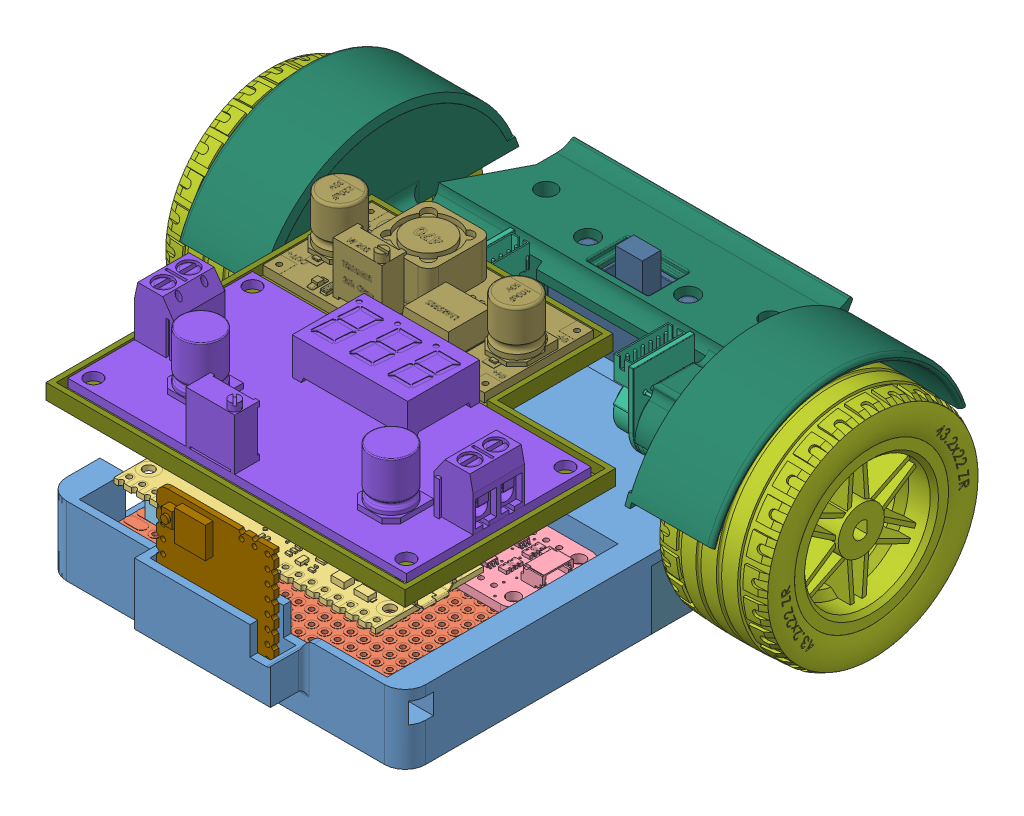
SolidWorks assembly Mini_Bot_V2.2, configuration Default. Lengths in mm.
Overall size (118.3 55.22 101.69).
22 component instances, 16 part files, 27 mates.
Components (placement in the parent):
- Bottom_Chasis-1: Bottom_Chasis [Default] at origin size (88 18.5 94)
- Main_Board-1: Main_Board [Default] at (58.2421 -7 43.2891) x (0 0 1) z (-1 0 0) size (44.13 18.54 60)
  - Universal_board_40x60mm.stp-1: Universal_board_40x60mm.stp [Default] at origin size (40 1.6 60)
  - Raspberry Pi Pico-R3-1: Raspberry Pi Pico-R3 [Default] at (-26.1161 13.25 58.3318) size (21 3.69 52.43)
  - LSM6DSOX acc gyro-1: LSM6DSOX acc gyro [Default] at (-48.9661 4 43.0918) x (0 0 -1) z (0 1 0) size (25.4 17.78 4.55)
  - PCB Terminal Block 2 DEG381-3.5.step-1: PCB Terminal Block 2 DEG381-3.5.step [Default] at (-44.2915 1.5 82.4428) x (1 0 0) z (0 1 0) size (7.4 7.4 12.2)
  - PCB Terminal Block 2 DEG381-3.5.step-2: PCB Terminal Block 2 DEG381-3.5.step [Default] at (-29.0999 1.5 82.5034) x (1 0 0) z (0 1 0) size (7.4 7.4 12.2)
- Wheel_Assembly-1: Wheel_Assembly [Default] at (-94.2185 0.6432 -267.7066) x (-1 0 0) z (0 0 -1) size (46.65 43 43)
  - N20_DC_Motor_and_Encoder-1: N20_DC_Motor_and_Encoder [Default] x (1 0 0) z (0 1 0) size (40.8 12 16)
  - Wheel-1: Wheel [Default] at (-142.6185 6.3568 -231.7066) x (-1 0 0) z (0 0 -1) size (22 43 43)
- Wheel_Assembly-2: Wheel_Assembly [Default] at (94.2185 0.6432 195.7066) size (46.65 43 43)
  - N20_DC_Motor_and_Encoder-1: N20_DC_Motor_and_Encoder [Default] x (1 0 0) z (0 1 0) size (40.8 12 16)
  - Wheel-1: Wheel [Default] at (-142.6185 6.3568 -231.7066) x (-1 0 0) z (0 0 -1) size (22 43 43)
- LM2596_Buck_Converter-4: LM2596_Buck_Converter [Default] at (0 19 11.25) x (-1 0 0) z (0 0 -1) size (66 17.65 36)
- Nicla Sense-1: Nicla Sense [Default] at (1.93 6.425 34.45) x (0 1 0) z (0 0 1) size (24.2 22.86 5.7)
- Switch-2: Switch [Default] at (0 2 -48.8943) x (-1 0 0) z (0 0 -1) size (30 20.5 11)
- 650_Tattu_LiPo_Battery_Pack-3: 650_Tattu_LiPo_Battery_Pack [Default] at (-33.7784 -10.1671 -18.6055) x (0 0 -1) z (1 0 0) size (30.31 11 69)
- LM2596_Mini_Buck_Converter-2: LM2596_Mini_Buck_Converter [Default] at (-11.4 19 -19.375) x (-1 0 0) z (0 0 -1) size (43.2 15.15 21.25)
- 1.5_Standoff-1: 1.5_Standoff [Default] at (-25.5141 2 -14.9861) size (6.93 15 6)
- Battery_Case-1: Battery_Case [Default] at (0 -11.5 -36.25) size (70 11.55 44.5)
- Switch_Motor_Top_Holder-1: Switch_Motor_Top_Holder [Default] at (0 17 -48.8943) x (-1 0 0) z (0 0 -1) size (104.09 38.72 52.86)
- Top_Chasis-1: Top_Chasis [Default] at (0 17 11.5) x (-1 0 0) z (0 0 -1) size (70 3 63.5)
Mates (geometry in assembly coordinates):
- Coincident1: coincident aligned: plane of Wheel_Assembly-1/N20_DC_Motor_and_Encoder-1 through (26.5 2 -36) normal (0 -1 0); plane of Wheel_Assembly-2/N20_DC_Motor_and_Encoder-1 through (-26.5 2 -36) normal (0 -1 0)
- Distance3: distance = 25 mm anti-aligned: plane of Wheel_Assembly-1/N20_DC_Motor_and_Encoder-1 through (12.5 7 -36) normal (-1 0 0); plane of Wheel_Assembly-2/N20_DC_Motor_and_Encoder-1 through (-12.5 7 -36) normal (1 0 0)
- Coincident3: coincident anti-aligned: plane of Bottom_Chasis-1 through (0 2 0) normal (0 1 0); plane of Wheel_Assembly-1/N20_DC_Motor_and_Encoder-1 through (26.5 2 -36) normal (0 -1 0)
- Coincident4: coincident anti-aligned: plane of Bottom_Chasis-1 through (0 2 0) normal (0 1 0); plane of Switch-2 through (0 2 -48.8943) normal (0 -1 0)
- Parallel3: parallel aligned: plane of Bottom_Chasis-1 through (0 2 -56) normal (0 0 -1); plane of Switch-2 through (12.25 14.5 -54.3943) normal (0 0 -1)
- Coincident10: coincident: point of Bottom_Chasis-1; unknown of Switch-2
- Distance4: distance = 2.5 mm anti-aligned: plane of Bottom_Chasis-1 through (84.3584 -9.5 31.5) normal (0 1 0); plane of Main_Board-1/Universal_board_40x60mm.stp-1 through (-35.9297 -7 33.563) normal (0 -1 0)
- Coincident12: coincident anti-aligned: plane of Bottom_Chasis-1 through (0 2 0) normal (0 1 0); plane of 1.5_Standoff-1 through (-25.5141 2 -14.9861) normal (0 -1 0)
- Distance5: distance = 2 mm anti-aligned: plane of 1.5_Standoff-1 through (-25.5141 17 -14.9861) normal (0 1 0); plane of LM2596_Buck_Converter-4 through (0 19 11.25) normal (0 -1 0)
- Coincident15: coincident aligned: plane of LM2596_Buck_Converter-4 through (0 19 11.25) normal (0 -1 0); plane of LM2596_Mini_Buck_Converter-2 through (-11.4 19 -19.375) normal (0 -1 0)
- Coincident16: coincident anti-aligned: plane of Bottom_Chasis-1 through (0 0 0) normal (0 -1 0); plane of Battery_Case-1 through (0 0 -36.25) normal (0 1 0)
- Coincident17: coincident anti-aligned: plane of Bottom_Chasis-1 through (84.3584 0 -16.5) normal (0 0 -1); plane of Battery_Case-1 through (-35 0 -16.5) normal (0 0 1)
- Coincident18: coincident aligned: plane of Bottom_Chasis-1 through (-35 2 0) normal (-1 0 0); plane of Battery_Case-1 through (-35 0 -16.5) normal (-1 0 0)
- Distance7: distance = 1.5 mm aligned: plane of Wheel_Assembly-1/N20_DC_Motor_and_Encoder-1 through (42.1 7 -42) normal (0 0 -1); plane of Bottom_Chasis-1 through (0 2 -43.5) normal (0 0 -1)
- Concentric1: concentric anti-aligned: cylinder of Switch-2 through (9.75 16 -48.8943) axis (0 -1 0) radius 1.65; cylinder of Switch_Motor_Top_Holder-1 through (9.75 3 -48.8943) axis (0 1 0) radius 2.025
- Concentric2: concentric anti-aligned: cylinder of Switch-2 through (-9.75 16 -48.8943) axis (0 -1 0) radius 1.65; cylinder of Switch_Motor_Top_Holder-1 through (-9.75 2 -48.8943) axis (0 1 0) radius 2.025
- Coincident25: coincident anti-aligned: plane of Wheel_Assembly-1/N20_DC_Motor_and_Encoder-1 through (26.5 12 -36) normal (0 1 0); plane of Switch_Motor_Top_Holder-1 through (0 12 -32.6834) normal (0 -1 0)
- Coincident26: coincident aligned: plane of LM2596_Buck_Converter-4 through (-33 20.6 29.25) normal (-1 0 0); plane of LM2596_Mini_Buck_Converter-2 through (-33 20.7 -30) normal (-1 0 0)
- Distance10: distance = 1 mm anti-aligned: plane of Top_Chasis-1 through (0 18 11.5) normal (0 1 0); plane of LM2596_Buck_Converter-4 through (0 19 11.25) normal (0 -1 0)
- Distance11: distance = 2 mm anti-aligned: plane of LM2596_Mini_Buck_Converter-2 through (10.2 20.7 -8.75) normal (0 0 1); plane of LM2596_Buck_Converter-4 through (33 20.6 -6.75) normal (0 0 -1)
- Distance12: distance = 1 mm anti-aligned: plane of Top_Chasis-1 through (0 20 -31) normal (0 0 1); plane of LM2596_Mini_Buck_Converter-2 through (10.2 20.7 -30) normal (0 0 -1)
- Distance13: distance = 1 mm anti-aligned: plane of Top_Chasis-1 through (-34 20 11.5) normal (1 0 0); plane of LM2596_Mini_Buck_Converter-2 through (-33 20.7 -30) normal (-1 0 0)
- Coincident32: coincident aligned: plane of Bottom_Chasis-1 through (-35 2 0) normal (-1 0 0); plane of Top_Chasis-1 through (-35 20 11.5) normal (-1 0 0)
- Coincident33: coincident aligned: plane of Bottom_Chasis-1 through (84.3584 0 31.5) normal (0 0 1); plane of Top_Chasis-1 through (0 20 31.5) normal (0 0 1)
- Coincident34: coincident anti-aligned: plane of Bottom_Chasis-1 through (15.25 -5 30) normal (0 1 0); plane of Nicla Sense-1 through (-9.5 -5 34.45) normal (0 -1 0)
- Distance14: distance = 0.25 mm anti-aligned: plane of Bottom_Chasis-1 through (-9.75 -30.526 31.5) normal (1 0 0); plane of Nicla Sense-1 through (-9.5 17.85 34.45) normal (-1 0 0)
- Distance15: distance = 0.5 mm anti-aligned: plane of Nicla Sense-1 through (-5.7 -1.25 32) normal (0 0 -1); plane of Bottom_Chasis-1 through (84.3584 0 31.5) normal (0 0 1)
